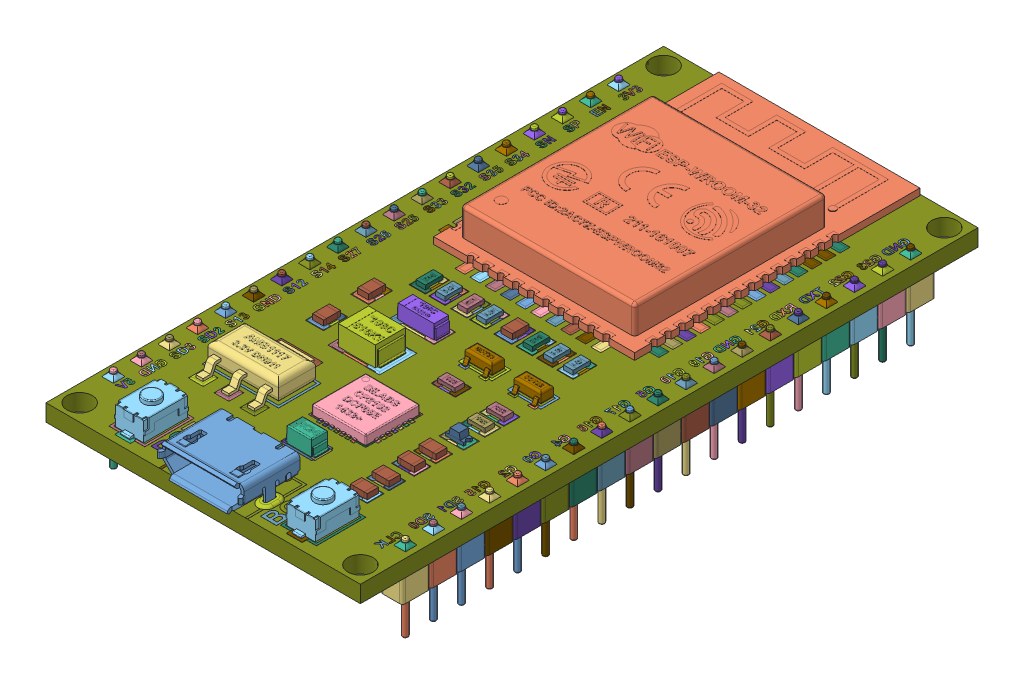
SolidWorks assembly PCB_ESP32-38Pines, configuration Default. Lengths in mm. (continued)
Components (placement in the parent): (continued)
- PCB_ESP32-38Pines.step-1: PCB_ESP32-38Pines.step [Default] at origin size (28 10.12 55.48) (continued)
  - PCB_ESP32-38Pines (v2~recovered)-254.step-1: PCB_ESP32-38Pines (v2~recovered)-254.step [Default] at origin size (0.74 0.01 0.67)
  - PCB_ESP32-38Pines (v2~recovered)-255.step-1: PCB_ESP32-38Pines (v2~recovered)-255.step [Default] at origin size (0.72 0.01 0.48)
  - PCB_ESP32-38Pines (v2~recovered)-256.step-1: PCB_ESP32-38Pines (v2~recovered)-256.step [Default] at origin size (0.72 0.01 0.48)
  - PCB_ESP32-38Pines (v2~recovered)-257.step-1: PCB_ESP32-38Pines (v2~recovered)-257.step [Default] at origin size (0.72 0.01 0.64)
  - PCB_ESP32-38Pines (v2~recovered)-258.step-1: PCB_ESP32-38Pines (v2~recovered)-258.step [Default] at origin size (0.72 0.01 0.48)
  - PCB_ESP32-38Pines (v2~recovered)-259.step-1: PCB_ESP32-38Pines (v2~recovered)-259.step [Default] at origin size (0.72 0.01 0.6)
  - PCB_ESP32-38Pines (v2~recovered)-260.step-1: PCB_ESP32-38Pines (v2~recovered)-260.step [Default] at origin size (0.74 0.01 0.67)
  - PCB_ESP32-38Pines (v2~recovered)-261.step-1: PCB_ESP32-38Pines (v2~recovered)-261.step [Default] at origin size (0.72 0.01 0.48)
  - PCB_ESP32-38Pines (v2~recovered)-262.step-1: PCB_ESP32-38Pines (v2~recovered)-262.step [Default] at origin size (0.74 0.01 0.67)
  - PCB_ESP32-38Pines (v2~recovered)-263.step-1: PCB_ESP32-38Pines (v2~recovered)-263.step [Default] at origin size (0.72 0.01 0.51)
  - PCB_ESP32-38Pines (v2~recovered)-264.step-1: PCB_ESP32-38Pines (v2~recovered)-264.step [Default] at origin size (0.72 0.01 0.48)
  - PCB_ESP32-38Pines (v2~recovered)-265.step-1: PCB_ESP32-38Pines (v2~recovered)-265.step [Default] at origin size (0.74 0.01 0.58)
  - PCB_ESP32-38Pines (v2~recovered)-266.step-1: PCB_ESP32-38Pines (v2~recovered)-266.step [Default] at origin size (0.72 0.01 0.6)
  - PCB_ESP32-38Pines (v2~recovered)-267.step-1: PCB_ESP32-38Pines (v2~recovered)-267.step [Default] at origin size (0.72 0.01 0.65)
  - PCB_ESP32-38Pines (v2~recovered)-268.step-1: PCB_ESP32-38Pines (v2~recovered)-268.step [Default] at origin size (1.43 0.01 1.14)
  - PCB_ESP32-38Pines (v2~recovered)-269.step-1: PCB_ESP32-38Pines (v2~recovered)-269.step [Default] at origin size (1.48 0.01 1.39)
  - PCB_ESP32-38Pines (v2~recovered)-270.step-1: PCB_ESP32-38Pines (v2~recovered)-270.step [Default] at origin size (1.43 0.01 1.29)
  - PCB_ESP32-38Pines (v2~recovered)-271.step-1: PCB_ESP32-38Pines (v2~recovered)-271.step [Default] at origin size (0.71 0.01 0.5)
  - PCB_ESP32-38Pines (v2~recovered)-272.step-1: PCB_ESP32-38Pines (v2~recovered)-272.step [Default] at origin size (0.74 0.01 0.58)
  - PCB_ESP32-38Pines (v2~recovered)-273.step-1: PCB_ESP32-38Pines (v2~recovered)-273.step [Default] at origin size (0.72 0.01 0.48)
  - PCB_ESP32-38Pines (v2~recovered)-274.step-1: PCB_ESP32-38Pines (v2~recovered)-274.step [Default] at origin size (0.74 0.01 0.67)
  - PCB_ESP32-38Pines (v2~recovered)-275.step-1: PCB_ESP32-38Pines (v2~recovered)-275.step [Default] at origin size (0.74 0.01 0.67)
  - PCB_ESP32-38Pines (v2~recovered)-276.step-1: PCB_ESP32-38Pines (v2~recovered)-276.step [Default] at origin size (0.71 0.01 0.47)
  - PCB_ESP32-38Pines (v2~recovered)-277.step-1: PCB_ESP32-38Pines (v2~recovered)-277.step [Default] at origin size (0.74 0.01 0.67)
  - PCB_ESP32-38Pines (v2~recovered)-278.step-1: PCB_ESP32-38Pines (v2~recovered)-278.step [Default] at origin size (0.73 0.01 0.48)
  - PCB_ESP32-38Pines (v2~recovered)-279.step-1: PCB_ESP32-38Pines (v2~recovered)-279.step [Default] at origin size (0.72 0.01 0.57)
  - PCB_ESP32-38Pines (v2~recovered)-280.step-1: PCB_ESP32-38Pines (v2~recovered)-280.step [Default] at origin size (0.74 0.01 0.67)
  - PCB_ESP32-38Pines (v2~recovered)-281.step-1: PCB_ESP32-38Pines (v2~recovered)-281.step [Default] at origin size (0.72 0.01 0.6)
  - PCB_ESP32-38Pines (v2~recovered)-282.step-1: PCB_ESP32-38Pines (v2~recovered)-282.step [Default] at origin size (0.72 0.01 0.48)
  - PCB_ESP32-38Pines (v2~recovered)-283.step-1: PCB_ESP32-38Pines (v2~recovered)-283.step [Default] at origin size (0.74 0.01 0.67)
  - PCB_ESP32-38Pines (v2~recovered)-284.step-1: PCB_ESP32-38Pines (v2~recovered)-284.step [Default] at origin size (0.73 0.01 0.48)
  - PCB_ESP32-38Pines (v2~recovered)-285.step-1: PCB_ESP32-38Pines (v2~recovered)-285.step [Default] at origin size (0.72 0.01 0.54)
  - PCB_ESP32-38Pines (v2~recovered)-286.step-1: PCB_ESP32-38Pines (v2~recovered)-286.step [Default] at origin size (0.74 0.01 0.58)
  - PCB_ESP32-38Pines (v2~recovered)-287.step-1: PCB_ESP32-38Pines (v2~recovered)-287.step [Default] at origin size (0.72 0.01 0.48)
  - PCB_ESP32-38Pines (v2~recovered)-288.step-1: PCB_ESP32-38Pines (v2~recovered)-288.step [Default] at origin size (0.73 0.01 0.48)
  - PCB_ESP32-38Pines (v2~recovered)-289.step-1: PCB_ESP32-38Pines (v2~recovered)-289.step [Default] at origin size (0.74 0.01 0.58)
  - PCB_ESP32-38Pines (v2~recovered)-290.step-1: PCB_ESP32-38Pines (v2~recovered)-290.step [Default] at origin size (0.73 0.01 0.48)
  - PCB_ESP32-38Pines (v2~recovered)-291.step-1: PCB_ESP32-38Pines (v2~recovered)-291.step [Default] at origin size (0.72 0.01 0.48)
  - PCB_ESP32-38Pines (v2~recovered)-292.step-1: PCB_ESP32-38Pines (v2~recovered)-292.step [Default] at origin size (0.74 0.01 0.58)
  - PCB_ESP32-38Pines (v2~recovered)-293.step-1: PCB_ESP32-38Pines (v2~recovered)-293.step [Default] at origin size (0.72 0.01 0.6)
  - PCB_ESP32-38Pines (v2~recovered)-294.step-1: PCB_ESP32-38Pines (v2~recovered)-294.step [Default] at origin size (0.72 0.01 0.31)
  - PCB_ESP32-38Pines (v2~recovered)-295.step-1: PCB_ESP32-38Pines (v2~recovered)-295.step [Default] at origin size (0.74 0.01 0.58)
  - PCB_ESP32-38Pines (v2~recovered)-296.step-1: PCB_ESP32-38Pines (v2~recovered)-296.step [Default] at origin size (0.74 0.01 0.67)
  - PCB_ESP32-38Pines (v2~recovered)-297.step-1: PCB_ESP32-38Pines (v2~recovered)-297.step [Default] at origin size (0.72 0.01 0.67)
  - PCB_ESP32-38Pines (v2~recovered)-298.step-1: PCB_ESP32-38Pines (v2~recovered)-298.step [Default] at origin size (1.5 0.02 1.5)
  - PCB_ESP32-38Pines (v2~recovered)-299.step-1: PCB_ESP32-38Pines (v2~recovered)-299.step [Default] at origin size (1.5 0.02 1.5)
  - PCB_ESP32-38Pines (v2~recovered)-300.step-1: PCB_ESP32-38Pines (v2~recovered)-300.step [Default] at origin size (1.4 0.02 2.05)
  - PCB_ESP32-38Pines (v2~recovered)-301.step-1: PCB_ESP32-38Pines (v2~recovered)-301.step [Default] at origin size (1.4 0.02 2.05)
  - PCB_ESP32-38Pines (v2~recovered)-302.step-1: PCB_ESP32-38Pines (v2~recovered)-302.step [Default] at origin size (3.32 0.1 3.3)
  - PCB_ESP32-38Pines (v2~recovered)-303.step-1: PCB_ESP32-38Pines (v2~recovered)-303.step [Default] at origin size (3.07 0.1 3.59)
  - PCB_ESP32-38Pines (v2~recovered)-304.step-1: PCB_ESP32-38Pines (v2~recovered)-304.step [Default] at origin size (15.55 0.1 10.25)
  - PCB_ESP32-38Pines (v2~recovered)-305.step-1: PCB_ESP32-38Pines (v2~recovered)-305.step [Default] at origin size (4.35 0.1 1.93)
  - PCB_ESP32-38Pines (v2~recovered)-306.step-1: PCB_ESP32-38Pines (v2~recovered)-306.step [Default] at origin size (8.67 0.1 4.03)
  - PCB_ESP32-38Pines (v2~recovered)-307.step-1: PCB_ESP32-38Pines (v2~recovered)-307.step [Default] at origin size (5.34 0.1 3.33)
  - PCB_ESP32-38Pines (v2~recovered)-308.step-1: PCB_ESP32-38Pines (v2~recovered)-308.step [Default] at origin size (1.7 0.01 1.9)
  - PCB_ESP32-38Pines (v2~recovered)-309.step-1: PCB_ESP32-38Pines (v2~recovered)-309.step [Default] at origin size (0.77 0.01 0.51)
  - PCB_ESP32-38Pines (v2~recovered)-310.step-1: PCB_ESP32-38Pines (v2~recovered)-310.step [Default] at origin size (1.07 0.01 2.5)
  - PCB_ESP32-38Pines (v2~recovered)-311.step-1: PCB_ESP32-38Pines (v2~recovered)-311.step [Default] at origin size (1.91 0.01 2.51)
  - PCB_ESP32-38Pines (v2~recovered)-312.step-1: PCB_ESP32-38Pines (v2~recovered)-312.step [Default] at origin size (3.55 0.01 4.29)
  - PCB_ESP32-38Pines (v2~recovered)-313.step-1: PCB_ESP32-38Pines (v2~recovered)-313.step [Default] at origin size (1.71 0.01 1.9)
  - PCB_ESP32-38Pines (v2~recovered)-314.step-1: PCB_ESP32-38Pines (v2~recovered)-314.step [Default] at origin size (1.65 0.01 1.86)
  - PCB_ESP32-38Pines (v2~recovered)-315.step-1: PCB_ESP32-38Pines (v2~recovered)-315.step [Default] at origin size (1.71 0.01 1.9)
  - PCB_ESP32-38Pines (v2~recovered)-316.step-1: PCB_ESP32-38Pines (v2~recovered)-316.step [Default] at origin size (3.94 0.01 4.29)
  - PCB_ESP32-38Pines (v2~recovered)-317.step-1: PCB_ESP32-38Pines (v2~recovered)-317.step [Default] at origin size (0.48 0.01 1.81)
  - PCB_ESP32-38Pines (v2~recovered)-318.step-1: PCB_ESP32-38Pines (v2~recovered)-318.step [Default] at origin size (1.18 0.01 1.86)
  - PCB_ESP32-38Pines (v2~recovered)-319.step-1: PCB_ESP32-38Pines (v2~recovered)-319.step [Default] at origin size (0.48 0.01 2.51)
  - PCB_ESP32-38Pines (v2~recovered)-320.step-1: PCB_ESP32-38Pines (v2~recovered)-320.step [Default] at origin size (3.8 0.01 4.44)
  - PCB_ESP32-38Pines (v2~recovered)-321.step-1: PCB_ESP32-38Pines (v2~recovered)-321.step [Default] at origin size (1.7 0.01 1.9)
  - PCB_ESP32-38Pines (v2~recovered)-322.step-1: PCB_ESP32-38Pines (v2~recovered)-322.step [Default] at origin size (1.87 0.01 1.9)
  - PCB_ESP32-38Pines (v2~recovered)-323.step-1: PCB_ESP32-38Pines (v2~recovered)-323.step [Default] at origin size (0.48 0.01 0.44)
  - PCB_ESP32-38Pines (v2~recovered)-324.step-1: PCB_ESP32-38Pines (v2~recovered)-324.step [Default] at origin size (4.1 0.01 4.29)
  - PCB_ESP32-38Pines (v2~recovered)-325.step-1: PCB_ESP32-38Pines (v2~recovered)-325.step [Default] at origin size (0.68 0.03 1.46)
  - PCB_ESP32-38Pines (v2~recovered)-326.step-1: PCB_ESP32-38Pines (v2~recovered)-326.step [Default] at origin size (1.6 0.03 0.72)
  - PCB_ESP32-38Pines (v2~recovered)-327.step-1: PCB_ESP32-38Pines (v2~recovered)-327.step [Default] at origin size (1.6 0.03 0.72)
  - PCB_ESP32-38Pines (v2~recovered)-328.step-1: PCB_ESP32-38Pines (v2~recovered)-328.step [Default] at origin size (1.46 0.03 0.68)
  - PCB_ESP32-38Pines (v2~recovered)-329.step-1: PCB_ESP32-38Pines (v2~recovered)-329.step [Default] at origin size (1.46 0.03 0.68)
  - PCB_ESP32-38Pines (v2~recovered)-330.step-1: PCB_ESP32-38Pines (v2~recovered)-330.step [Default] at origin size (1.46 0.03 0.68)
  - PCB_ESP32-38Pines (v2~recovered)-331.step-1: PCB_ESP32-38Pines (v2~recovered)-331.step [Default] at origin size (1.46 0.03 0.68)
  - PCB_ESP32-38Pines (v2~recovered)-332.step-1: PCB_ESP32-38Pines (v2~recovered)-332.step [Default] at origin size (0.65 0.03 0.53)
  - PCB_ESP32-38Pines (v2~recovered)-333.step-1: PCB_ESP32-38Pines (v2~recovered)-333.step [Default] at origin size (0.68 0.03 1.46)
  - PCB_ESP32-38Pines (v2~recovered)-334.step-1: PCB_ESP32-38Pines (v2~recovered)-334.step [Default] at origin size (0.6 0.03 1.5)
  - PCB_ESP32-38Pines (v2~recovered)-335.step-1: PCB_ESP32-38Pines (v2~recovered)-335.step [Default] at origin size (0.6 0.03 1.5)
  - PCB_ESP32-38Pines (v2~recovered)-336.step-1: PCB_ESP32-38Pines (v2~recovered)-336.step [Default] at origin size (1.4 0.03 0.61)
  - PCB_ESP32-38Pines (v2~recovered)-337.step-1: PCB_ESP32-38Pines (v2~recovered)-337.step [Default] at origin size (0.6 0.03 1.65)
  - PCB_ESP32-38Pines (v2~recovered)-338.step-1: PCB_ESP32-38Pines (v2~recovered)-338.step [Default] at origin size (1.32 0.03 1.33)
  - PCB_ESP32-38Pines (v2~recovered)-339.step-1: PCB_ESP32-38Pines (v2~recovered)-339.step [Default] at origin size (0.44 0.03 1.01)
  - PCB_ESP32-38Pines (v2~recovered)-340.step-1: PCB_ESP32-38Pines (v2~recovered)-340.step [Default] at origin size (0.44 0.03 1.01)
  - PCB_ESP32-38Pines (v2~recovered)-341.step-1: PCB_ESP32-38Pines (v2~recovered)-341.step [Default] at origin size (1.32 0.03 1.33)
  - PCB_ESP32-38Pines (v2~recovered)-342.step-1: PCB_ESP32-38Pines (v2~recovered)-342.step [Default] at origin size (0.6 0.03 1.65)
  - PCB_ESP32-38Pines (v2~recovered)-343.step-1: PCB_ESP32-38Pines (v2~recovered)-343.step [Default] at origin size (1.4 0.03 0.61)
  - PCB_ESP32-38Pines (v2~recovered)-344.step-1: PCB_ESP32-38Pines (v2~recovered)-344.step [Default] at origin size (0.6 0.03 1.5)
  - PCB_ESP32-38Pines (v2~recovered)-345.step-1: PCB_ESP32-38Pines (v2~recovered)-345.step [Default] at origin size (0.6 0.03 1.5)
  - PCB_ESP32-38Pines (v2~recovered)-346.step-1: PCB_ESP32-38Pines (v2~recovered)-346.step [Default] at origin size (0.68 0.03 1.46)
  - PCB_ESP32-38Pines (v2~recovered)-347.step-1: PCB_ESP32-38Pines (v2~recovered)-347.step [Default] at origin size (0.65 0.03 0.53)
  - PCB_ESP32-38Pines (v2~recovered)-348.step-1: PCB_ESP32-38Pines (v2~recovered)-348.step [Default] at origin size (1.46 0.03 0.68)
  - PCB_ESP32-38Pines (v2~recovered)-349.step-1: PCB_ESP32-38Pines (v2~recovered)-349.step [Default] at origin size (1.46 0.03 0.68)
  - PCB_ESP32-38Pines (v2~recovered)-350.step-1: PCB_ESP32-38Pines (v2~recovered)-350.step [Default] at origin size (1.46 0.03 0.68)
  - PCB_ESP32-38Pines (v2~recovered)-351.step-1: PCB_ESP32-38Pines (v2~recovered)-351.step [Default] at origin size (1.46 0.03 0.68)
  - PCB_ESP32-38Pines (v2~recovered)-352.step-1: PCB_ESP32-38Pines (v2~recovered)-352.step [Default] at origin size (1.6 0.03 0.72)
  - PCB_ESP32-38Pines (v2~recovered)-353.step-1: PCB_ESP32-38Pines (v2~recovered)-353.step [Default] at origin size (1.6 0.03 0.72)
  - PCB_ESP32-38Pines (v2~recovered)-354.step-1: PCB_ESP32-38Pines (v2~recovered)-354.step [Default] at origin size (0.68 0.03 1.46)
  - PCB_ESP32-38Pines (v2~recovered)-355.step-1: PCB_ESP32-38Pines (v2~recovered)-355.step [Default] at origin size (0.74 0.03 1.4)
  - PCB_ESP32-38Pines (v2~recovered)-356.step-1: PCB_ESP32-38Pines (v2~recovered)-356.step [Default] at origin size (1.31 0.03 3.33)
  - PCB_ESP32-38Pines (v2~recovered)-357.step-1: PCB_ESP32-38Pines (v2~recovered)-357.step [Default] at origin size (1 0.03 1.92)
  - PCB_ESP32-38Pines (v2~recovered)-358.step-1: PCB_ESP32-38Pines (v2~recovered)-358.step [Default] at origin size (1.46 0.03 0.68)
  - PCB_ESP32-38Pines (v2~recovered)-359.step-1: PCB_ESP32-38Pines (v2~recovered)-359.step [Default] at origin size (1.46 0.03 0.68)
  - PCB_ESP32-38Pines (v2~recovered)-360.step-1: PCB_ESP32-38Pines (v2~recovered)-360.step [Default] at origin size (1.6 0.03 0.72)
  - PCB_ESP32-38Pines (v2~recovered)-361.step-1: PCB_ESP32-38Pines (v2~recovered)-361.step [Default] at origin size (1.46 0.03 0.68)
  - PCB_ESP32-38Pines (v2~recovered)-362.step-1: PCB_ESP32-38Pines (v2~recovered)-362.step [Default] at origin size (0.65 0.03 0.53)
  - PCB_ESP32-38Pines (v2~recovered)-363.step-1: PCB_ESP32-38Pines (v2~recovered)-363.step [Default] at origin size (0.65 0.03 0.53)
  - PCB_ESP32-38Pines (v2~recovered)-364.step-1: PCB_ESP32-38Pines (v2~recovered)-364.step [Default] at origin size (0.68 0.03 1.46)
  - PCB_ESP32-38Pines (v2~recovered)-365.step-1: PCB_ESP32-38Pines (v2~recovered)-365.step [Default] at origin size (0.6 0.03 1.5)
  - PCB_ESP32-38Pines (v2~recovered)-366.step-1: PCB_ESP32-38Pines (v2~recovered)-366.step [Default] at origin size (0.6 0.03 1.5)
  - PCB_ESP32-38Pines (v2~recovered)-367.step-1: PCB_ESP32-38Pines (v2~recovered)-367.step [Default] at origin size (1.4 0.03 0.61)
  - PCB_ESP32-38Pines (v2~recovered)-368.step-1: PCB_ESP32-38Pines (v2~recovered)-368.step [Default] at origin size (1.32 0.03 1.33)
  - PCB_ESP32-38Pines (v2~recovered)-369.step-1: PCB_ESP32-38Pines (v2~recovered)-369.step [Default] at origin size (0.44 0.03 1.01)
  - PCB_ESP32-38Pines (v2~recovered)-370.step-1: PCB_ESP32-38Pines (v2~recovered)-370.step [Default] at origin size (0.44 0.03 1.01)
  - PCB_ESP32-38Pines (v2~recovered)-371.step-1: PCB_ESP32-38Pines (v2~recovered)-371.step [Default] at origin size (0.44 0.03 1.01)
  - PCB_ESP32-38Pines (v2~recovered)-372.step-1: PCB_ESP32-38Pines (v2~recovered)-372.step [Default] at origin size (3.75 0.03 2.04)
  - PCB_ESP32-38Pines (v2~recovered)-373.step-1: PCB_ESP32-38Pines (v2~recovered)-373.step [Default] at origin size (1.4 0.03 0.61)
  - PCB_ESP32-38Pines (v2~recovered)-374.step-1: PCB_ESP32-38Pines (v2~recovered)-374.step [Default] at origin size (0.6 0.03 1.5)
  - PCB_ESP32-38Pines (v2~recovered)-375.step-1: PCB_ESP32-38Pines (v2~recovered)-375.step [Default] at origin size (0.6 0.03 1.5)
  - PCB_ESP32-38Pines (v2~recovered)-376.step-1: PCB_ESP32-38Pines (v2~recovered)-376.step [Default] at origin size (0.68 0.03 1.46)
  - PCB_ESP32-38Pines (v2~recovered)-377.step-1: PCB_ESP32-38Pines (v2~recovered)-377.step [Default] at origin size (0.65 0.03 0.53)
  - PCB_ESP32-38Pines (v2~recovered)-378.step-1: PCB_ESP32-38Pines (v2~recovered)-378.step [Default] at origin size (0.65 0.03 0.53)
  - PCB_ESP32-38Pines (v2~recovered)-379.step-1: PCB_ESP32-38Pines (v2~recovered)-379.step [Default] at origin size (1.46 0.03 0.68)
  - PCB_ESP32-38Pines (v2~recovered)-380.step-1: PCB_ESP32-38Pines (v2~recovered)-380.step [Default] at origin size (1.6 0.03 0.72)
  - PCB_ESP32-38Pines (v2~recovered)-381.step-1: PCB_ESP32-38Pines (v2~recovered)-381.step [Default] at origin size (1.46 0.03 0.68)
  - PCB_ESP32-38Pines (v2~recovered)-382.step-1: PCB_ESP32-38Pines (v2~recovered)-382.step [Default] at origin size (1.46 0.03 0.68)
  - PCB_ESP32-38Pines (v2~recovered)-383.step-1: PCB_ESP32-38Pines (v2~recovered)-383.step [Default] at origin size (1 0.03 1.92)
  - PCB_ESP32-38Pines (v2~recovered)-384.step-1: PCB_ESP32-38Pines (v2~recovered)-384.step [Default] at origin size (1.31 0.03 3.33)
  - PCB_ESP32-38Pines (v2~recovered)-385.step-1: PCB_ESP32-38Pines (v2~recovered)-385.step [Default] at origin size (0.74 0.03 1.4)
  - PCB_ESP32-38Pines (v2~recovered)-386.step-1: PCB_ESP32-38Pines (v2~recovered)-386.step [Default] at origin size (1.4 0.2 2.05)
  - PCB_ESP32-38Pines (v2~recovered)-387.step-1: PCB_ESP32-38Pines (v2~recovered)-387.step [Default] at origin size (1 0.2 1)
  - PCB_ESP32-38Pines (v2~recovered)-388.step-1: PCB_ESP32-38Pines (v2~recovered)-388.step [Default] at origin size (1 0.2 1)
  - PCB_ESP32-38Pines (v2~recovered)-389.step-1: PCB_ESP32-38Pines (v2~recovered)-389.step [Default] at origin size (1.4 0.2 2.05)
  - PCB_ESP32-38Pines (v2~recovered)-390.step-1: PCB_ESP32-38Pines (v2~recovered)-390.step [Default] at origin size (0.6 0.02 0.34)
  - PCB_ESP32-38Pines (v2~recovered)-391.step-1: PCB_ESP32-38Pines (v2~recovered)-391.step [Default] at origin size (0.6 0.02 0.34)
  - PCB_ESP32-38Pines (v2~recovered)-392.step-1: PCB_ESP32-38Pines (v2~recovered)-392.step [Default] at origin size (0.34 0.02 0.6)
  - PCB_ESP32-38Pines (v2~recovered)-393.step-1: PCB_ESP32-38Pines (v2~recovered)-393.step [Default] at origin size (0.6 0.02 0.34)
  - PCB_ESP32-38Pines (v2~recovered)-394.step-1: PCB_ESP32-38Pines (v2~recovered)-394.step [Default] at origin size (0.6 0.02 0.34)
  - PCB_ESP32-38Pines (v2~recovered)-395.step-1: PCB_ESP32-38Pines (v2~recovered)-395.step [Default] at origin size (0.34 0.02 0.6)
  - PCB_ESP32-38Pines (v2~recovered)-396.step-1: PCB_ESP32-38Pines (v2~recovered)-396.step [Default] at origin size (0.34 0.02 0.6)
  - PCB_ESP32-38Pines (v2~recovered)-397.step-1: PCB_ESP32-38Pines (v2~recovered)-397.step [Default] at origin size (1.54 0.02 0.9)
  - PCB_ESP32-38Pines (v2~recovered)-398.step-1: PCB_ESP32-38Pines (v2~recovered)-398.step [Default] at origin size (1.54 0.02 0.9)
  - PCB_ESP32-38Pines (v2~recovered)-399.step-1: PCB_ESP32-38Pines (v2~recovered)-399.step [Default] at origin size (1.54 0.02 0.9)
  - PCB_ESP32-38Pines (v2~recovered)-400.step-1: PCB_ESP32-38Pines (v2~recovered)-400.step [Default] at origin size (0.9 0.02 1.54)
  - PCB_ESP32-38Pines (v2~recovered)-401.step-1: PCB_ESP32-38Pines (v2~recovered)-401.step [Default] at origin size (0.9 0.02 1.54)
  - PCB_ESP32-38Pines (v2~recovered)-402.step-1: PCB_ESP32-38Pines (v2~recovered)-402.step [Default] at origin size (0.9 0.02 1.54)
  - PCB_ESP32-38Pines (v2~recovered)-403.step-1: PCB_ESP32-38Pines (v2~recovered)-403.step [Default] at origin size (1.54 0.02 0.9)
  - PCB_ESP32-38Pines (v2~recovered)-404.step-1: PCB_ESP32-38Pines (v2~recovered)-404.step [Default] at origin size (1.54 0.02 0.9)
  - PCB_ESP32-38Pines (v2~recovered)-405.step-1: PCB_ESP32-38Pines (v2~recovered)-405.step [Default] at origin size (1.54 0.02 0.9)
  - PCB_ESP32-38Pines (v2~recovered)-406.step-1: PCB_ESP32-38Pines (v2~recovered)-406.step [Default] at origin size (1.54 0.02 0.9)
  - PCB_ESP32-38Pines (v2~recovered)-407.step-1: PCB_ESP32-38Pines (v2~recovered)-407.step [Default] at origin size (1.54 0.02 0.9)
  - PCB_ESP32-38Pines (v2~recovered)-408.step-1: PCB_ESP32-38Pines (v2~recovered)-408.step [Default] at origin size (1.54 0.02 0.9)
  - PCB_ESP32-38Pines (v2~recovered)-409.step-1: PCB_ESP32-38Pines (v2~recovered)-409.step [Default] at origin size (1.54 0.02 0.9)
  - PCB_ESP32-38Pines (v2~recovered)-410.step-1: PCB_ESP32-38Pines (v2~recovered)-410.step [Default] at origin size (0.9 0.02 1.54)
  - PCB_ESP32-38Pines (v2~recovered)-411.step-1: PCB_ESP32-38Pines (v2~recovered)-411.step [Default] at origin size (0.9 0.02 1.54)
  - PCB_ESP32-38Pines (v2~recovered)-412.step-1: PCB_ESP32-38Pines (v2~recovered)-412.step [Default] at origin size (1.54 0.02 0.9)
  - PCB_ESP32-38Pines (v2~recovered)-413.step-1: PCB_ESP32-38Pines (v2~recovered)-413.step [Default] at origin size (1.54 0.02 0.9)
  - PCB_ESP32-38Pines (v2~recovered)-414.step-1: PCB_ESP32-38Pines (v2~recovered)-414.step [Default] at origin size (1.54 0.02 0.9)
  - PCB_ESP32-38Pines (v2~recovered)-415.step-1: PCB_ESP32-38Pines (v2~recovered)-415.step [Default] at origin size (1.54 0.02 0.9)
  - PCB_ESP32-38Pines (v2~recovered)-416.step-1: PCB_ESP32-38Pines (v2~recovered)-416.step [Default] at origin size (0.34 0.02 0.6)
  - PCB_ESP32-38Pines (v2~recovered)-417.step-1: PCB_ESP32-38Pines (v2~recovered)-417.step [Default] at origin size (0.34 0.02 0.6)
  - PCB_ESP32-38Pines (v2~recovered)-418.step-1: PCB_ESP32-38Pines (v2~recovered)-418.step [Default] at origin size (0.6 0.02 0.34)
  - PCB_ESP32-38Pines (v2~recovered)-419.step-1: PCB_ESP32-38Pines (v2~recovered)-419.step [Default] at origin size (0.34 0.02 0.6)
  - PCB_ESP32-38Pines (v2~recovered)-420.step-1: PCB_ESP32-38Pines (v2~recovered)-420.step [Default] at origin size (0.34 0.02 0.6)
  - PCB_ESP32-38Pines (v2~recovered)-421.step-1: PCB_ESP32-38Pines (v2~recovered)-421.step [Default] at origin size (0.6 0.02 0.34)
  - PCB_ESP32-38Pines (v2~recovered)-422.step-1: PCB_ESP32-38Pines (v2~recovered)-422.step [Default] at origin size (0.6 0.02 0.34)
  - PCB_ESP32-38Pines (v2~recovered)-423.step-1: PCB_ESP32-38Pines (v2~recovered)-423.step [Default] at origin size (0.6 0.02 0.34)
  - PCB_ESP32-38Pines (v2~recovered)-424.step-1: PCB_ESP32-38Pines (v2~recovered)-424.step [Default] at origin size (0.34 0.02 0.6)
  - PCB_ESP32-38Pines (v2~recovered)-425.step-1: PCB_ESP32-38Pines (v2~recovered)-425.step [Default] at origin size (0.34 0.02 0.6)
  - PCB_ESP32-38Pines (v2~recovered)-426.step-1: PCB_ESP32-38Pines (v2~recovered)-426.step [Default] at origin size (0.6 0.02 0.34)
  - PCB_ESP32-38Pines (v2~recovered)-427.step-1: PCB_ESP32-38Pines (v2~recovered)-427.step [Default] at origin size (0.6 0.02 0.34)
  - PCB_ESP32-38Pines (v2~recovered)-428.step-1: PCB_ESP32-38Pines (v2~recovered)-428.step [Default] at origin size (0.34 0.02 0.6)
  - PCB_ESP32-38Pines (v2~recovered)-429.step-1: PCB_ESP32-38Pines (v2~recovered)-429.step [Default] at origin size (0.34 0.02 0.6)
  - PCB_ESP32-38Pines (v2~recovered)-430.step-1: PCB_ESP32-38Pines (v2~recovered)-430.step [Default] at origin size (1.54 0.02 0.9)
  - PCB_ESP32-38Pines (v2~recovered)-431.step-1: PCB_ESP32-38Pines (v2~recovered)-431.step [Default] at origin size (1.54 0.02 0.9)
  - PCB_ESP32-38Pines (v2~recovered)-432.step-1: PCB_ESP32-38Pines (v2~recovered)-432.step [Default] at origin size (1.54 0.02 0.9)
  - PCB_ESP32-38Pines (v2~recovered)-433.step-1: PCB_ESP32-38Pines (v2~recovered)-433.step [Default] at origin size (0.9 0.02 1.54)
  - PCB_ESP32-38Pines (v2~recovered)-434.step-1: PCB_ESP32-38Pines (v2~recovered)-434.step [Default] at origin size (0.9 0.02 1.54)
  - PCB_ESP32-38Pines (v2~recovered)-435.step-1: PCB_ESP32-38Pines (v2~recovered)-435.step [Default] at origin size (0.9 0.02 1.54)
  - PCB_ESP32-38Pines (v2~recovered)-436.step-1: PCB_ESP32-38Pines (v2~recovered)-436.step [Default] at origin size (1.54 0.02 0.9)
  - PCB_ESP32-38Pines (v2~recovered)-437.step-1: PCB_ESP32-38Pines (v2~recovered)-437.step [Default] at origin size (1.54 0.02 0.9)
  - PCB_ESP32-38Pines (v2~recovered)-438.step-1: PCB_ESP32-38Pines (v2~recovered)-438.step [Default] at origin size (1.54 0.02 0.9)
  - PCB_ESP32-38Pines (v2~recovered)-439.step-1: PCB_ESP32-38Pines (v2~recovered)-439.step [Default] at origin size (1.54 0.02 0.9)
  - PCB_ESP32-38Pines (v2~recovered)-440.step-1: PCB_ESP32-38Pines (v2~recovered)-440.step [Default] at origin size (1.54 0.02 0.9)
  - PCB_ESP32-38Pines (v2~recovered)-441.step-1: PCB_ESP32-38Pines (v2~recovered)-441.step [Default] at origin size (1.54 0.02 0.9)
  - PCB_ESP32-38Pines (v2~recovered)-442.step-1: PCB_ESP32-38Pines (v2~recovered)-442.step [Default] at origin size (1.54 0.02 0.9)
  - PCB_ESP32-38Pines (v2~recovered)-443.step-1: PCB_ESP32-38Pines (v2~recovered)-443.step [Default] at origin size (0.9 0.02 1.54)
  - PCB_ESP32-38Pines (v2~recovered)-444.step-1: PCB_ESP32-38Pines (v2~recovered)-444.step [Default] at origin size (0.9 0.02 1.54)
  - PCB_ESP32-38Pines (v2~recovered)-445.step-1: PCB_ESP32-38Pines (v2~recovered)-445.step [Default] at origin size (1.54 0.02 0.9)
  - PCB_ESP32-38Pines (v2~recovered)-446.step-1: PCB_ESP32-38Pines (v2~recovered)-446.step [Default] at origin size (1.54 0.02 0.9)
  - PCB_ESP32-38Pines (v2~recovered)-447.step-1: PCB_ESP32-38Pines (v2~recovered)-447.step [Default] at origin size (1.54 0.02 0.9)
  - PCB_ESP32-38Pines (v2~recovered)-448.step-1: PCB_ESP32-38Pines (v2~recovered)-448.step [Default] at origin size (1.54 0.02 0.9)
  - PCB_ESP32-38Pines (v2~recovered)-449.step-1: PCB_ESP32-38Pines (v2~recovered)-449.step [Default] at origin size (0.34 0.02 0.6)
  - PCB_ESP32-38Pines (v2~recovered)-450.step-1: PCB_ESP32-38Pines (v2~recovered)-450.step [Default] at origin size (0.6 0.02 0.34)
  - PCB_ESP32-38Pines (v2~recovered)-451.step-1: PCB_ESP32-38Pines (v2~recovered)-451.step [Default] at origin size (0.6 0.02 0.34)
  - PCB_ESP32-38Pines (v2~recovered)-452.step-1: PCB_ESP32-38Pines (v2~recovered)-452.step [Default] at origin size (0.34 0.02 0.6)
  - PCB_ESP32-38Pines (v2~recovered)-453.step-1: PCB_ESP32-38Pines (v2~recovered)-453.step [Default] at origin size (0.34 0.02 0.6)
  - PCB_ESP32-38Pines (v2~recovered)-454.step-1: PCB_ESP32-38Pines (v2~recovered)-454.step [Default] at origin size (0.6 0.02 0.34)
  - PCB_ESP32-38Pines (v2~recovered)-455.step-1: PCB_ESP32-38Pines (v2~recovered)-455.step [Default] at origin size (0.6 0.02 0.34)
